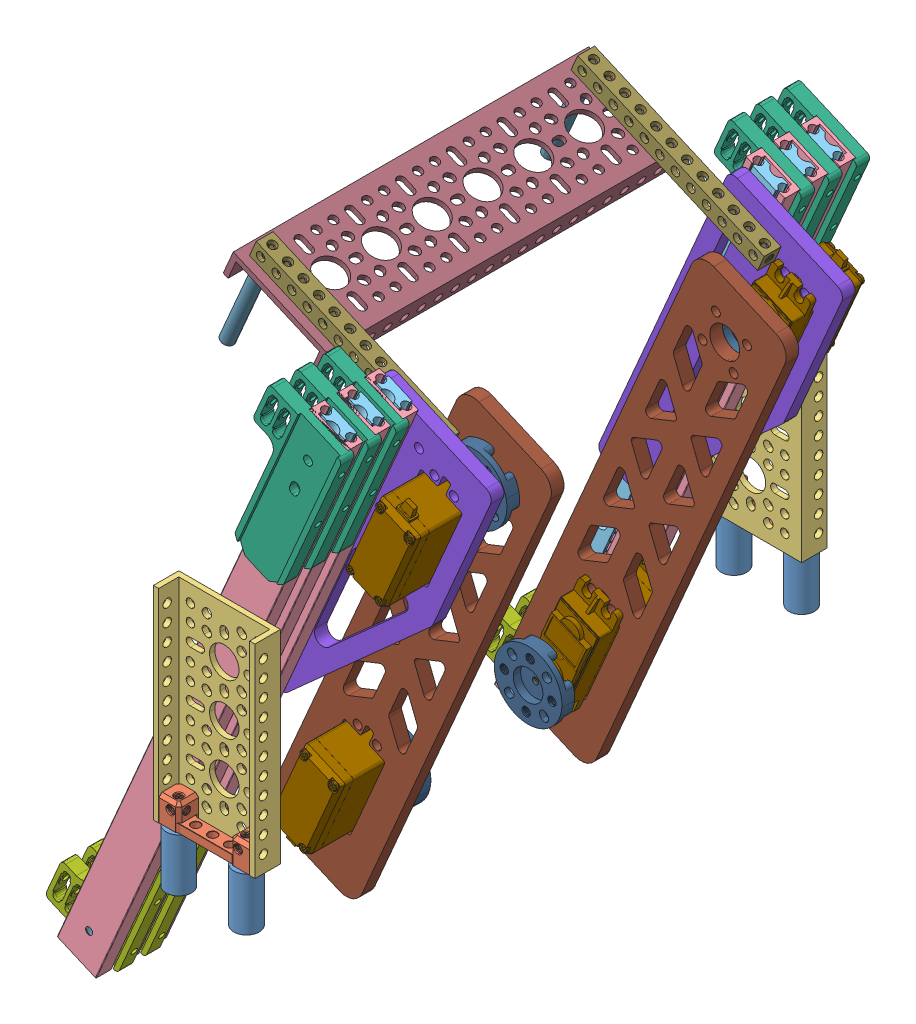
SolidWorks assembly Outtake Sub-Assembly League Meet 2, configuration Default. Lengths in mm.
Overall size (188.36 300.4 277.38).
54 component instances, 14 part files, 63 mates.
Components (placement in the parent):
- 25mm spacer-1: 25mm spacer [Default] at (131.527 64.1625 -130.2749) x (0.98393 0 0.178554) z (-0.178554 0 0.98393) size (12 25 12)
- 25mm spacer-2: 25mm spacer [Default] at (99.527 64.1625 -130.2749) x (0.999949 0 -0.010072) z (0.010072 0 0.999949) size (12 25 12)
- 25mm spacer-4: 25mm spacer [Default] at (131.527 64.1625 132.0751) x (0.974267 0 -0.225397) z (0.225397 0 0.974267) size (12 25 12)
- 25mm spacer-6: 25mm spacer [Default] at (99.527 64.1625 132.0751) x (0.894277 0 -0.447515) z (0.447515 0 0.894277) size (12 25 12)
- dual block.step-1: dual block.step [Default] at (115.527 93.1625 -146.2749) x (0 0 -1) z (0 -1 0) size (9.5 43 12)
- dual block.step-2: dual block.step [Default] at (115.527 93.0375 148.0751) x (0 0 1) z (0 -1 0) size (9.5 43 12)
- 3 Hole Low-Side U Channel 96mm.step-1: 3 Hole Low-Side U Channel 96mm.step [Default] at (94.027 89.0375 148.0751) x (0 0 1) z (-1 0 0) size (12 96 48)
- 3 Hole Low-Side U Channel 96mm.step-2: 3 Hole Low-Side U Channel 96mm.step [Default] at (137.027 89.1625 -146.2749) x (0 0 -1) z (1 0 0) size (12 96 48)
- SAR230 Moveable-1: SAR230 Moveable [Default] at (34.4642 1.8723 -116.8999) x (0 0 1) z (0.396729 0.917936 0) size (8.01 20 300)
  - SAR230_3-1: SAR230_3 [Default] at (5.2 -3.95 0) size (7.4 20 300)
  - SAR230_5-1: SAR230_5 [Default] at (0.0108 0 0) size (5.81 12.1 300)
- LK_Drawer-Slide-Pulley-Insert_v20220723_LH-1: LK_Drawer-Slide-Pulley-Insert_v20220723_LH [Default] at (159.0363 274.8529 -108.5891) x (-0.396729 -0.917936 0) z (0 0 1) size (76.2 37.5 6.35)
- LK_Drawer-Slide-Pulley-Insert_v20220723-1: LK_Drawer-Slide-Pulley-Insert_v20220723 [1_RightHand] at (40.0177 -0.5279 -108.5891) x (0.396729 0.917936 0) z (0 0 1) size (76.2 37.5 6.35)
- LK_Drawer-Slide-Pulley-Insert_v20220723-2: LK_Drawer-Slide-Pulley-Insert_v20220723 [1_RightHand] at (40.0177 -0.5279 -95.5783) x (0.396729 0.917936 0) z (0 0 1) size (76.2 37.5 6.35)
- LK_Drawer-Slide-Pulley-Insert_v20220723_LH-3: LK_Drawer-Slide-Pulley-Insert_v20220723_LH [Default] at (159.0363 274.8529 -95.5783) x (-0.396729 -0.917936 0) z (0 0 1) size (76.2 37.5 6.35)
- SAR230 Moveable-2: SAR230 Moveable [Default] at (34.4642 1.8723 -103.8891) x (0 0 1) z (0.396729 0.917936 0) size (8.01 20 300)
  - SAR230_3-1: SAR230_3 [Default] at (5.2 -3.95 0) size (7.4 20 300)
  - SAR230_5-1: SAR230_5 [Default] at (0.0108 0 0) size (5.81 12.1 300)
- SAR230 Moveable-4: SAR230 Moveable [Default] at (34.4642 1.8723 -90.8783) x (0 0 1) z (0.396729 0.917936 0) size (8.01 20 300)
  - SAR230_3-1: SAR230_3 [Default] at (5.2 -3.95 0) size (7.4 20 300)
  - SAR230_5-1: SAR230_5 [Default] at (0.0108 0 0) size (5.81 12.1 300)
- LK_Drawer-Slide-Pulley-Insert_v20220723_LH-7: LK_Drawer-Slide-Pulley-Insert_v20220723_LH [Default] at (159.0363 274.8529 -121.5999) x (-0.396729 -0.917936 0) z (0 0 1) size (76.2 37.5 6.35)
- SAR230 Moveable-6: SAR230 Moveable [Default] at (45.5712 -2.9281 105.6892) x (0 0 -1) z (0.396729 0.917936 0) size (8.01 20 300)
  - SAR230_3-1: SAR230_3 [Default] at (5.2 -3.95 0) size (7.4 20 300)
  - SAR230_5-1: SAR230_5 [Default] at (0.0108 0 0) size (5.81 12.1 300)
- LK_Drawer-Slide-Pulley-Insert_v20220723_LH-10: LK_Drawer-Slide-Pulley-Insert_v20220723_LH [Default] at (159.0363 274.8529 96.0309) x (-0.396729 -0.917936 0) z (0 0 1) size (76.2 37.5 6.35)
- SAR230 Moveable-7: SAR230 Moveable [Default] at (45.5712 -2.9281 92.6784) x (0 0 -1) z (0.396729 0.917936 0) size (8.01 20 300)
  - SAR230_3-1: SAR230_3 [Default] at (5.2 -3.95 0) size (7.4 20 300)
  - SAR230_5-1: SAR230_5 [Default] at (0.0108 0 0) size (5.81 12.1 300)
- LK_Drawer-Slide-Pulley-Insert_v20220723_LH-11: LK_Drawer-Slide-Pulley-Insert_v20220723_LH [Default] at (159.0363 274.8529 122.0525) x (-0.396729 -0.917936 0) z (0 0 1) size (76.2 37.5 6.35)
- LK_Drawer-Slide-Pulley-Insert_v20220723_LH-12: LK_Drawer-Slide-Pulley-Insert_v20220723_LH [Default] at (159.0363 274.8529 109.0417) x (-0.396729 -0.917936 0) z (0 0 1) size (76.2 37.5 6.35)
- SAR230 Moveable-8: SAR230 Moveable [Default] at (45.5712 -2.9281 118.7001) x (0 0 -1) z (0.396729 0.917936 0) size (8.01 20 300)
  - SAR230_3-1: SAR230_3 [Default] at (5.2 -3.95 0) size (7.4 20 300)
  - SAR230_5-1: SAR230_5 [Default] at (0.0108 0 0) size (5.81 12.1 300)
- LK_Drawer-Slide-Pulley-Insert_v20220723-6: LK_Drawer-Slide-Pulley-Insert_v20220723 [1_RightHand] at (40.0177 -0.5279 109.0392) x (0.396729 0.917936 0) z (0 0 1) size (76.2 37.5 6.35)
- LK_Drawer-Slide-Pulley-Insert_v20220723-7: LK_Drawer-Slide-Pulley-Insert_v20220723 [1_RightHand] at (40.0177 -0.5279 96.0284) x (0.396729 0.917936 0) z (0 0 1) size (76.2 37.5 6.35)
- Servo Mounting Plate Iteration 2-1: Servo Mounting Plate Iteration 2 [Default] at (126.3062 199.1232 -85.0674) x (0.917936 -0.396729 0) z (-0.396729 -0.917936 0) size (59.48 6 159)
- Servo Mounting Plate Iteration 2-2: Servo Mounting Plate Iteration 2 [Default] at (126.3062 199.1232 80.8676) x (0.917936 -0.396729 0) z (-0.396729 -0.917936 0) size (59.48 6 159)
- servo.step-1: servo.step [Default] at (169.9694 222.8149 69.6676) x (-0.396729 -0.917936 0) z (0 0 -1) size (54.3 20 43.9)
- servo.step-2: servo.step [Default] at (169.9694 222.8149 -67.8674) x (-0.396729 -0.917936 0) z (0 0 1) size (54.3 20 43.9)
- 1908-0025-0032.step-1: 1908-0025-0032.step [Default] at (173.8772 231.8565 59.3639) x (-0.197005 0.980402 0) z (0.980402 0.197005 0) size (31.98 8 31.98)
- Bar ARm-1: Bar ARm [Default] at (135.7912 143.7347 59.3676) x (-0.917936 0.396729 0) z (-0.396729 -0.917936 0) size (48 6 240)
- Bar ARm-2: Bar ARm [Default] at (135.7912 143.7347 -57.5674) x (0.917936 -0.396729 0) z (-0.396729 -0.917936 0) size (48 6 240)
- 1908-0025-0032.step-2: 1908-0025-0032.step [Default] at (173.8772 231.8565 -65.5674) x (-0.197005 0.980402 0) z (0.980402 0.197005 0) size (31.98 8 31.98)
- servo.step-3: servo.step [Default] at (106.3539 75.6238 42.1676) x (0.396729 0.917936 0) z (0 0 -1) size (54.3 20 43.9)
- servo.step-5: servo.step [Default] at (106.3539 75.6238 -40.3674) x (0.396729 0.917936 0) z (0 0 1) size (54.3 20 43.9)
- Assem3^Outtake Sub-Assembly League Meet 2-1: Assem3^Outtake Sub-Assembly League Meet 2 [Default] at origin (virtual)
- 1908-0025-0032.step-3: 1908-0025-0032.step [Default] at (102.4462 66.5822 39.8676) x (0.276712 0.960953 0) z (-0.960953 0.276712 0) size (31.98 8 31.98)
- 1908-0025-0032.step-5: 1908-0025-0032.step [Default] at (102.4462 66.5822 -38.0674) x (-0.082356 -0.996603 0) z (-0.996603 0.082356 0) size (31.98 8 31.98)
- 12 hole beam.step-1: 12 hole beam.step [Default] at (86.994 289.6483 76.8676) x (0.396729 0.917936 0) z (0 0 -1) size (8 96.01 8)
- 12 hole beam.step-3: 12 hole beam.step [Default] at (86.994 289.6483 -75.0674) x (-0.396729 -0.917936 0) z (0 0 1) size (8 96.01 8)
- 6 Hole Low-Side U Channel 168mm.step-1: 6 Hole Low-Side U Channel 168mm.step [Default] at (70.8369 266.1281 -83.1324) x (-0.396729 -0.917936 0) z (-0.917936 0.396729 0) size (12 168 48)
- 1501-0006-0430.step-1: 1501-0006-0430.step [Default] at (75.8856 263.9461 -75.0674) x (0.917936 -0.396729 0) z (0 0 1) size (5.95 43.01 5.95)
- 1501-0006-0430.step-2: 1501-0006-0430.step [Default] at (75.8856 263.9461 76.8676) x (-0.046972 0.020301 -0.99869) z (0.916733 -0.396209 -0.051171) size (5.95 43.01 5.95)
Mates (geometry in assembly coordinates):
- Coincident13: coincident anti-aligned: plane of SAR230 Moveable-1/SAR230_5-1 through (153.6663 277.1737 -111.0891) normal (0 0 1); plane of LK_Drawer-Slide-Pulley-Insert_v20220723_LH-1 through (159.0363 274.8529 -111.0891) normal (0 0 -1)
- Coincident14: coincident anti-aligned: plane of SAR230 Moveable-1/SAR230_5-1 through (153.6663 277.1737 -111.0891) normal (0 0 1); plane of LK_Drawer-Slide-Pulley-Insert_v20220723-1 through (40.0177 -0.5279 -111.0891) normal (0 0 -1)
- Concentric13: concentric aligned: circle of SAR230 Moveable-1/SAR230_5-1; cylinder of LK_Drawer-Slide-Pulley-Insert_v20220723-1 through (45.9686 13.2411 -111.0891) axis (0 0 1) radius 2.125
- Parallel3: parallel aligned: plane of SAR230 Moveable-1/SAR230_3-1 through (149.8569 278.8202 -118.7999) normal (-0.917936 0.396729 0); plane of LK_Drawer-Slide-Pulley-Insert_v20220723-1 through (28.5435 4.4312 -106.0891) normal (-0.917936 0.396729 0)
- Concentric14: concentric aligned: circle of SAR230 Moveable-1/SAR230_5-1; cylinder of LK_Drawer-Slide-Pulley-Insert_v20220723_LH-1 through (153.0853 261.0838 -111.0891) axis (0 0 1) radius 2.125
- Parallel4: parallel anti-aligned: plane of SAR230 Moveable-1/SAR230_3-1 through (149.8569 278.8202 -118.7999) normal (-0.917936 0.396729 0); plane of LK_Drawer-Slide-Pulley-Insert_v20220723_LH-1 through (170.5105 269.8938 -106.0891) normal (0.917936 -0.396729 0)
- Coincident17: coincident anti-aligned: plane of LK_Drawer-Slide-Pulley-Insert_v20220723_LH-3 through (159.0363 274.8529 -98.0783) normal (0 0 -1); plane of SAR230 Moveable-2/SAR230_5-1 through (153.6663 277.1737 -98.0783) normal (0 0 1)
- Coincident18: coincident anti-aligned: plane of LK_Drawer-Slide-Pulley-Insert_v20220723-2 through (40.0177 -0.5279 -98.0783) normal (0 0 -1); plane of SAR230 Moveable-2/SAR230_5-1 through (153.6663 277.1737 -98.0783) normal (0 0 1)
- Concentric15: concentric aligned: cylinder of LK_Drawer-Slide-Pulley-Insert_v20220723-2 through (45.9686 13.2411 -98.0783) axis (0 0 1) radius 2.125; circle of SAR230 Moveable-2/SAR230_5-1
- Parallel5: parallel aligned: plane of LK_Drawer-Slide-Pulley-Insert_v20220723-2 through (28.5435 4.4312 -93.0783) normal (-0.917936 0.396729 0); plane of SAR230 Moveable-2/SAR230_3-1 through (149.8569 278.8202 -105.7891) normal (-0.917936 0.396729 0)
- Concentric16: concentric aligned: cylinder of LK_Drawer-Slide-Pulley-Insert_v20220723_LH-3 through (153.0853 261.0838 -98.0783) axis (0 0 1) radius 2.125; circle of SAR230 Moveable-2/SAR230_5-1
- Parallel6: parallel anti-aligned: plane of LK_Drawer-Slide-Pulley-Insert_v20220723_LH-3 through (170.5105 269.8938 -93.0783) normal (0.917936 -0.396729 0); plane of SAR230 Moveable-2/SAR230_3-1 through (149.8569 278.8202 -105.7891) normal (-0.917936 0.396729 0)
- Coincident19: coincident anti-aligned: plane of LK_Drawer-Slide-Pulley-Insert_v20220723_LH-1 through (159.0363 274.8529 -106.0891) normal (0 0 1); plane of SAR230 Moveable-2/SAR230_3-1 through (167.9403 271.0046 -106.0891) normal (0 0 -1)
- Concentric17: concentric aligned: cylinder of SAR230 Moveable-1/SAR230_5-1 through (99.527 137.1625 -111.0891) axis (0 0 1) radius 1.621; cylinder of SAR230 Moveable-2/SAR230_5-1 through (99.527 137.1625 -98.0783) axis (0 0 1) radius 1.621
- Coincident24: coincident anti-aligned: plane of LK_Drawer-Slide-Pulley-Insert_v20220723_LH-3 through (159.0363 274.8529 -93.0783) normal (0 0 1); plane of SAR230 Moveable-4/SAR230_3-1 through (167.9403 271.0046 -93.0783) normal (0 0 -1)
- Concentric22: concentric aligned: cylinder of SAR230 Moveable-2/SAR230_5-1 through (99.527 137.1625 -98.0783) axis (0 0 1) radius 1.621; cylinder of SAR230 Moveable-4/SAR230_5-1 through (99.527 137.1625 -85.0674) axis (0 0 1) radius 1.621
- Coincident27: coincident aligned: plane of SAR230 Moveable-2/SAR230_3-1 through (149.8569 278.8202 -105.7891) normal (-0.917936 0.396729 0); plane of SAR230 Moveable-4/SAR230_3-1 through (149.8569 278.8202 -92.7783) normal (-0.917936 0.396729 0)
- Coincident28: coincident aligned: plane of SAR230 Moveable-1/SAR230_3-1 through (149.8569 278.8202 -118.7999) normal (-0.917936 0.396729 0); plane of SAR230 Moveable-4/SAR230_3-1 through (149.8569 278.8202 -92.7783) normal (-0.917936 0.396729 0)
- Concentric25: concentric aligned: circle of SAR230 Moveable-1/SAR230_3-1; cylinder of LK_Drawer-Slide-Pulley-Insert_v20220723_LH-7 through (153.0853 261.0838 -124.0999) axis (0 0 1) radius 2.125
- Parallel13: parallel anti-aligned: plane of SAR230 Moveable-1/SAR230_3-1 through (149.8569 278.8202 -118.7999) normal (-0.917936 0.396729 0); plane of LK_Drawer-Slide-Pulley-Insert_v20220723_LH-7 through (170.5105 269.8938 -119.0999) normal (0.917936 -0.396729 0)
- Coincident29: coincident anti-aligned: plane of SAR230 Moveable-1/SAR230_3-1 through (167.9403 271.0046 -119.0999) normal (0 0 -1); plane of LK_Drawer-Slide-Pulley-Insert_v20220723_LH-7 through (159.0363 274.8529 -119.0999) normal (0 0 1)
- Concentric26: concentric aligned: circle of SAR230 Moveable-4/SAR230_5-1; circle of Servo Mounting Plate Iteration 2-1
- Coincident30: coincident anti-aligned: plane of SAR230 Moveable-4/SAR230_5-1 through (153.6663 277.1737 -85.0674) normal (0 0 1); plane of Servo Mounting Plate Iteration 2-1 through (126.3062 199.1232 -85.0674) normal (0 0 -1)
- Concentric27: concentric anti-aligned: circle of SAR230 Moveable-4/SAR230_5-1; cylinder of Servo Mounting Plate Iteration 2-1 through (99.527 137.1625 -79.0674) axis (0 0 -1) radius 2.1
- Concentric77: concentric aligned: circle of servo.step-3; cylinder of 1908-0025-0032.step-3 through (102.4462 66.5822 59.6948) axis (0 0 -1) radius 7.01
- Coincident112: coincident anti-aligned: plane of servo.step-3 through (102.4462 66.5822 36.4676) normal (0 0 -1); plane of 1908-0025-0032.step-3 through (102.4462 66.5822 36.4676) normal (0 0 1)
- Coincident113: coincident anti-aligned: plane of dual block.step-1 through (137.027 93.1625 -124.7749) normal (0 0 1); plane of 3 Hole Low-Side U Channel 96mm.step-2 through (137.027 185.1625 -124.7749) normal (0 0 -1)
- Concentric80: concentric aligned: cylinder of 25mm spacer-1 through (131.527 89.1625 -130.2749) axis (0 -1 0) radius 6; circle of dual block.step-1
- Concentric81: concentric anti-aligned: circle of dual block.step-1; cylinder of 3 Hole Low-Side U Channel 96mm.step-2 through (131.527 97.1625 -132.2749) axis (0 0 1) radius 2
- Coincident114: coincident anti-aligned: plane of 25mm spacer-1 through (131.527 89.1625 -130.2749) normal (0 1 0); plane of dual block.step-1 through (115.527 89.1625 -147.5249) normal (0 -1 0)
- Coincident115: coincident anti-aligned: plane of dual block.step-1 through (94.027 93.1625 -124.7749) normal (-1 0 0); plane of 3 Hole Low-Side U Channel 96mm.step-2 through (94.027 79.3391 -134.2749) normal (1 0 0)
- Concentric82: concentric aligned: cylinder of 3 Hole Low-Side U Channel 96mm.step-2 through (99.527 137.1625 -132.2749) axis (0 0 1) radius 2; circle of SAR230 Moveable-1/SAR230_3-1
- Concentric83: concentric anti-aligned: circle of dual block.step-2; cylinder of 3 Hole Low-Side U Channel 96mm.step-1 through (99.527 97.0375 134.0751) axis (0 0 -1) radius 2
- Concentric84: concentric aligned: cylinder of 25mm spacer-4 through (131.527 89.1625 132.0751) axis (0 -1 0) radius 3; circle of dual block.step-2
- Parallel40: parallel aligned: plane of dual block.step-2 through (137.027 93.0375 126.5751) normal (1 0 0); plane of 3 Hole Low-Side U Channel 96mm.step-1 through (139.527 185.0375 126.5751) normal (1 0 0)
- Coincident117: coincident: plane of 25mm spacer-4 through (131.527 89.1625 132.0751) normal (0 1 0); line of dual block.step-2 through (129.027 89.1625 136.0751) axis (1 0 0)
- Coincident118: coincident anti-aligned: plane of dual block.step-2 through (94.027 93.0375 126.5751) normal (0 0 -1); plane of 3 Hole Low-Side U Channel 96mm.step-1 through (94.027 185.0375 126.5751) normal (0 0 1)
- Coincident119: coincident anti-aligned: plane of Bar ARm-2 through (135.7912 143.7347 -57.5674) normal (0 0 -1); plane of 1908-0025-0032.step-2 through (173.8772 231.8565 -57.5674) normal (0 0 1)
- Concentric86: concentric aligned: cylinder of Bar ARm-2 through (173.8772 231.8565 -51.5674) axis (0 0 -1) radius 7.1; cylinder of 1908-0025-0032.step-2 through (173.8772 231.8565 -57.5674) axis (0 0 -1) radius 15.99
- Concentric87: concentric aligned: circle of servo.step-2; cylinder of 1908-0025-0032.step-2 through (173.8772 231.8565 -12.3409) axis (0 0 -1) radius 4.99
- Coincident120: coincident anti-aligned: plane of servo.step-2 through (173.8772 231.8565 -62.1674) normal (0 0 1); plane of 1908-0025-0032.step-2 through (173.8772 231.8565 -62.1674) normal (0 0 -1)
- Concentric88: concentric anti-aligned: cylinder of Servo Mounting Plate Iteration 2-1 through (155.9041 202.7482 -79.0674) axis (0 0 -1) radius 2.1; circle of servo.step-2
- Parallel41: parallel aligned: plane of Servo Mounting Plate Iteration 2-1 through (85.5869 130.1146 -79.0674) normal (-0.917936 0.396729 0); plane of servo.step-2 through (150.6139 203.2371 -76.3674) normal (-0.917936 0.396729 0)
- Coincident122: coincident anti-aligned: plane of Servo Mounting Plate Iteration 2-1 through (126.3062 199.1232 -79.0674) normal (0 0 1); plane of servo.step-2 through (167.5957 195.8976 -79.0674) normal (0 0 -1)
- Concentric93: concentric aligned: circle of Bar ARm-1; cylinder of servo.step-3 through (101.3762 51.6296 53.3686) axis (0 0 -1) radius 2.25
- Parallel43: parallel aligned: plane of Bar ARm-1 through (110.2142 24.0609 53.3676) normal (0.917936 -0.396729 0); plane of servo.step-3 through (123.2497 89.5104 53.3676) normal (0.917936 -0.396729 0)
- Coincident124: coincident anti-aligned: plane of Bar ARm-1 through (135.7912 143.7347 53.3676) normal (0 0 -1); plane of servo.step-3 through (124.3325 95.7967 53.3676) normal (0 0 1)
- Concentric94: concentric aligned: circle of servo.step-5; cylinder of 1908-0025-0032.step-5 through (102.4462 66.5822 -30.0674) axis (0 0 -1) radius 15.99
- Coincident125: coincident anti-aligned: plane of servo.step-5 through (102.4462 66.5822 -34.6674) normal (0 0 1); plane of 1908-0025-0032.step-5 through (102.4462 66.5822 -34.6674) normal (0 0 -1)
- Parallel46: parallel aligned: plane of SAR230 Moveable-4/SAR230_3-1 through (149.8569 278.8202 -92.7783) normal (-0.917936 0.396729 0); plane of Bar ARm-2 through (66.1533 43.1039 -51.5674) normal (-0.917936 0.396729 0)
- Coincident135: coincident anti-aligned: plane of Servo Mounting Plate Iteration 2-2 through (126.3062 199.1232 80.8676) normal (0 0 -1); plane of 12 hole beam.step-1 through (90.6657 288.0614 80.8676) normal (0 0 1)
- Concentric102: concentric anti-aligned: cylinder of Servo Mounting Plate Iteration 2-2 through (167.7723 254.7362 86.8676) axis (0 0 -1) radius 2.1; cylinder of 12 hole beam.step-1 through (167.7723 254.7362 80.8676) axis (0 0 1) radius 2
- Concentric103: concentric anti-aligned: cylinder of Servo Mounting Plate Iteration 2-2 through (153.0853 261.0838 86.8676) axis (0 0 -1) radius 2.1; cylinder of 12 hole beam.step-1 through (153.0853 261.0838 80.8676) axis (0 0 1) radius 2
- Coincident137: coincident anti-aligned: plane of Servo Mounting Plate Iteration 2-1 through (126.3062 199.1232 -79.0674) normal (0 0 1); plane of 12 hole beam.step-3 through (90.6657 288.0614 -79.0674) normal (0 0 -1)
- Concentric104: concentric aligned: cylinder of Servo Mounting Plate Iteration 2-1 through (167.7723 254.7362 -79.0674) axis (0 0 -1) radius 2.1; cylinder of 12 hole beam.step-3 through (167.7723 254.7362 -79.0674) axis (0 0 -1) radius 2
- Concentric105: concentric aligned: cylinder of Servo Mounting Plate Iteration 2-1 through (153.0853 261.0838 -79.0674) axis (0 0 -1) radius 2.1; cylinder of 12 hole beam.step-3 through (153.0853 261.0838 -79.0674) axis (0 0 -1) radius 2
- Coincident138: coincident anti-aligned: plane of 12 hole beam.step-1 through (89.0788 284.3897 76.8676) normal (-0.396729 -0.917936 0); plane of 6 Hole Low-Side U Channel 168mm.step-1 through (122.1245 270.1074 84.8676) normal (0.396729 0.917936 0)
- Concentric106: concentric aligned: circle of 12 hole beam.step-1; circle of 6 Hole Low-Side U Channel 168mm.step-1
- Concentric107: concentric aligned: cylinder of 12 hole beam.step-1 through (117.9548 280.6247 76.8676) axis (0.396729 0.917936 0) radius 2; cylinder of 6 Hole Low-Side U Channel 168mm.step-1 through (110.8137 264.1019 76.8676) axis (0.396729 0.917936 0) radius 2
- Concentric108: concentric aligned: cylinder of 12 hole beam.step-3 through (85.407 285.9766 -75.0674) axis (-0.396729 -0.917936 0) radius 2; cylinder of 1501-0006-0430.step-1 through (84.4152 283.6817 -75.0674) axis (-0.396729 -0.917936 0) radius 2.975
- Coincident140: coincident aligned: circle of 6 Hole Low-Side U Channel 168mm.step-1; plane of 1501-0006-0430.step-1 through (84.4152 283.6817 -75.0674) normal (0.396729 0.917936 0)
- Concentric109: concentric anti-aligned: cylinder of 6 Hole Low-Side U Channel 168mm.step-1 through (81.4398 276.7972 76.8676) axis (0.396729 0.917936 0) radius 2; cylinder of 1501-0006-0430.step-2 through (84.4152 283.6817 76.8676) axis (-0.396729 -0.917936 0) radius 2.975
- Coincident141: coincident anti-aligned: plane of 6 Hole Low-Side U Channel 168mm.step-1 through (79.3666 285.8637 84.8676) normal (-0.396729 -0.917936 0); plane of 1501-0006-0430.step-2 through (84.4152 283.6817 76.8676) normal (0.396729 0.917936 0)
